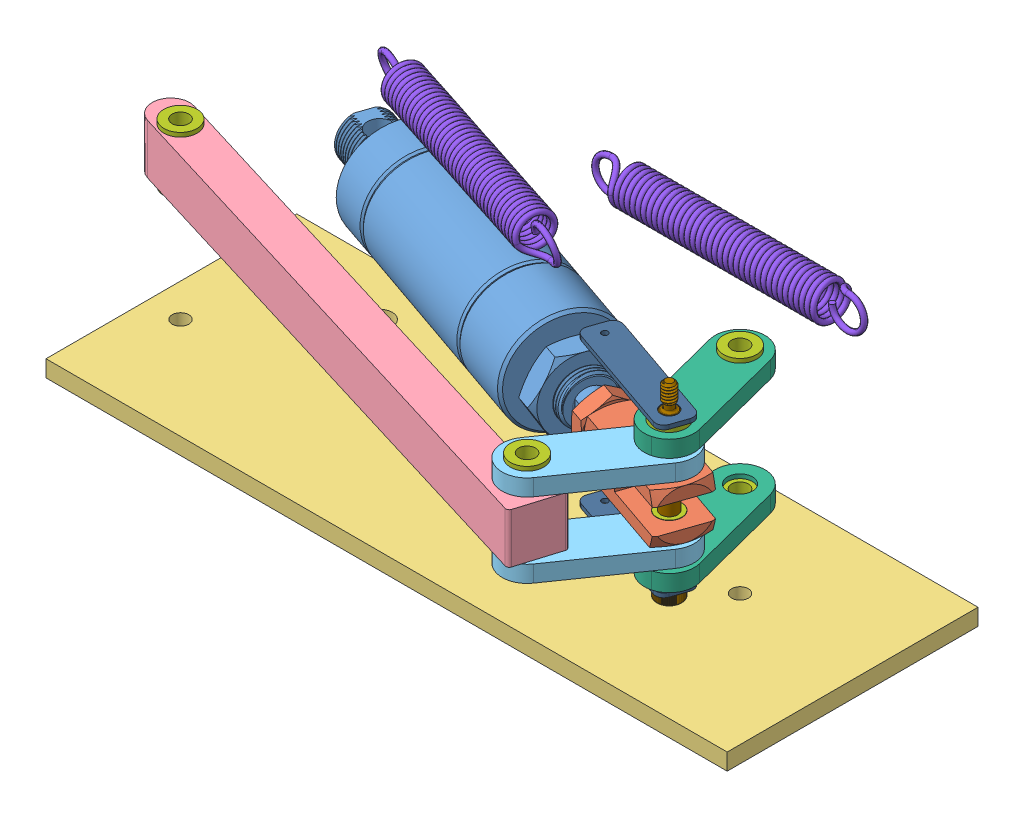
SolidWorks assembly Brake Assembly, configuration Default. Lengths in mm.
Overall size (538.69 101.29 156.86).
28 component instances, 10 part files, 54 mates.
Components (placement in the parent):
- Braking Piston-1: Braking Piston [Default] at (164.5211 173.4692 63.7009) x (-0.945257 0 -0.326326) z (0 -1 0) size (198.34 39.62 39.62) (flexible)
  - Piston for Brakes 6498K983-1: Piston for Brakes 6498K983 [6498K983] at (80.307 95.7083 111.838) size (166.18 39.62 39.62)
  - Brake Piston Rod Clevis 6498K44-1: Brake Piston Rod Clevis 6498K44 [6498K44] at (7.9351 95.7083 111.838) x (0 0 1) z (0 -1 0) size (22 51.06 19.05)
- Brake Mounting Bar-1: Brake Mounting Bar [Default] at (50.8149 0 -76.8043) size (538.69 6.35 114.9)
- Brake Bottom Bar-1: Brake Bottom Bar [Default] at (57.3167 52.1062 -68.9319) x (0.982053 0 0.188604) z (-0.188604 0 0.982053) size (214.1 19.05 36.15)
- Brake Bottom Short Linkage-1: Brake Bottom Short Linkage [Default] at (78.7603 44.1687 -113.4175) x (0.97252 0 0.23282) z (-0.23282 0 0.97252) size (33.27 6.35 55.41)
- Brake Bottom Short Linkage-2: Brake Bottom Short Linkage [Default] at (78.7603 72.7437 -113.4175) x (0.97252 0 0.23282) z (-0.23282 0 0.97252) size (33.27 6.35 55.41)
- Brake Short Top Short Linkage-1: Brake Short Top Short Linkage [Default] at (50.5741 36.2312 -34.9184) x (0.966151 0 -0.257976) z (0.257976 0 0.966151) size (19.38 6.35 56.68)
- Brake Short Top Short Linkage-2: Brake Short Top Short Linkage [Default] at (50.5741 80.6812 -34.9184) x (0.966151 0 -0.257976) z (0.257976 0 0.966151) size (19.38 6.35 56.68)
- Brakes Bronze Bushing-1: Brakes Bronze Bushing [6338K411] at (219.705 72.7437 -18.4994) x (-0.83291 0 -0.553408) z (-0.553408 0 0.83291) size (12.7 6.35 12.7)
- Brakes Bronze Bushing-2: Brakes Bronze Bushing [6338K411] at (219.705 50.5187 -18.4994) size (12.7 6.35 12.7)
- Brakes Bronze Bushing-3: Brakes Bronze Bushing [6338K411] at (197.4073 72.7437 13.5493) x (0.840037 0 0.542529) z (0.542529 0 -0.840037) size (12.7 6.35 12.7)
- Brakes Bronze Bushing-4: Brakes Bronze Bushing [6338K411] at (197.4073 50.5187 13.5493) x (0.999992 0 -0.00402) z (0.00402 0 0.999992) size (12.7 6.35 12.7)
- Brakes Bronze Bushing-5: Brakes Bronze Bushing [6338K411] at (219.705 80.6812 -18.4994) x (-0.837169 0 -0.546944) z (-0.546944 0 0.837169) size (12.7 6.35 12.7)
- Brakes Bronze Bushing-6: Brakes Bronze Bushing [6338K411] at (219.705 42.5812 -18.4994) size (12.7 6.35 12.7)
- Brakes Bronze Bushing-7: Brakes Bronze Bushing [6338K411] at (210.3103 34.6437 -54.9436) size (12.7 6.35 12.7)
- Brakes Bronze Bushing-8: Brakes Bronze Bushing [6338K411] at (219.705 88.6187 -18.4994) x (-0.891229 0 -0.453553) z (-0.453553 0 0.891229) size (12.7 6.35 12.7)
- Brakes Bronze Bushing-9: Brakes Bronze Bushing [6338K411] at (210.3103 88.6187 -54.9436) x (-0.837169 0 -0.546944) z (-0.546944 0 0.837169) size (12.7 6.35 12.7)
- Brakes Bronze Bushing-10: Brakes Bronze Bushing [6338K411] at (219.705 34.6437 -18.4994) x (0.965083 0 -0.261946) z (0.261946 0 0.965083) size (12.7 6.35 12.7)
- Brakes Bronze Bushing-12: Brakes Bronze Bushing [6338K411] at (12.7 50.5187 -38.7043) x (0.988051 0 -0.154127) z (0.154127 0 0.988051) size (12.7 6.35 12.7)
- Brakes Bronze Bushing-13: Brakes Bronze Bushing [6338K411] at (12.7 72.7437 -38.7043) x (-0.837169 0 -0.546944) z (-0.546944 0 0.837169) size (12.7 6.35 12.7)
- Brakes Bronze Bushing-14: Brakes Bronze Bushing [6338K411] at (197.4073 80.6812 13.5493) x (-0.983904 0 -0.178699) z (-0.178699 0 0.983904) size (12.7 6.35 12.7)
- Brakes Bronze Bushing-15: Brakes Bronze Bushing [6338K411] at (197.4073 42.5812 13.5493) size (12.7 6.35 12.7)
- Brakes Return Spring-1: Brakes Return Spring [9654K324] at (100.1802 92.2599 -61.7232) x (0.952226 -0.005044 0.305352) z (0.296812 0.250647 -0.921455) size (104.77 14.45 14.71)
- Brakes Return Spring-2: Brakes Return Spring [9654K324] at (140.1667 54.0208 -121.1624) size (104.77 14.45 14.71)
- Brakes Piston Head Pivot Bolt-1: Brakes Piston Head Pivot Bolt [91259A104] at (219.705 33.0562 -18.4994) x (-0.730056 0 -0.683388) z (-0.683388 0 0.730056) size (9.53 71.79 9.53)
- Brakes Brake Extensions-1: Brakes Brake Extensions [Default] at (179.7604 90.2062 -39.007) x (0.945257 0 0.326326) z (0.326326 0 -0.945257) size (50.8 1.59 12.7)
- Brakes Brake Extensions-2: Brakes Brake Extensions [Default] at (175.6161 33.0562 -27.0022) x (0.945257 0 0.326326) z (-0.326326 0 0.945257) size (50.8 1.59 12.7)
Mates (geometry in assembly coordinates):
- Coincident5: coincident aligned: plane of Brake Mounting Bar-1 through (0 6.35 0) normal (0 0 1); plane of assembly through (0 0 0) normal (0 0 1)
- Coincident6: coincident anti-aligned: plane of Brake Mounting Bar-1 through (50.8149 0 -76.8043) normal (0 -1 0); plane of assembly through (0 0 0) normal (0 1 0)
- Coincident7: coincident anti-aligned: plane of Brake Mounting Bar-1 through (0 6.35 -95.8543) normal (-1 0 0); plane of assembly through (0 0 0) normal (1 0 0)
- Concentric3: concentric anti-aligned: cylinder of Braking Piston-1/Piston for Brakes 6498K983-1 through (50.8149 71.1562 -76.8043) axis (0 -1 0) radius 4.7625; cylinder of Brake Mounting Bar-1 through (50.8149 0 -76.8043) axis (0 1 0) radius 4.7625
- Concentric4: concentric aligned: cylinder of Brake Mounting Bar-1 through (12.7 0 -38.7043) axis (0 1 0) radius 3.175; cylinder of Brake Bottom Bar-1 through (12.7 52.1062 -38.7043) axis (0 1 0) radius 4.7625
- Concentric5: concentric aligned: cylinder of Brake Bottom Short Linkage-2 through (219.705 79.0937 -18.4994) axis (0 -1 0) radius 4.7625; cylinder of Braking Piston-1/Brake Piston Rod Clevis 6498K44-1 through (219.705 71.1562 -18.4994) axis (0 -1 0) radius 4.826
- Concentric6: concentric aligned: cylinder of Braking Piston-1/Brake Piston Rod Clevis 6498K44-1 through (219.705 71.1562 -18.4994) axis (0 -1 0) radius 4.826; cylinder of Brake Bottom Short Linkage-1 through (219.705 50.5187 -18.4994) axis (0 -1 0) radius 4.7625
- Concentric7: concentric anti-aligned: cylinder of Brake Bottom Bar-1 through (197.4073 52.1062 13.5493) axis (0 1 0) radius 4.7625; cylinder of Brake Bottom Short Linkage-1 through (197.4073 50.5187 13.5493) axis (0 -1 0) radius 4.7625
- Concentric8: concentric anti-aligned: cylinder of Brake Bottom Bar-1 through (197.4073 52.1062 13.5493) axis (0 1 0) radius 4.7625; cylinder of Brake Bottom Short Linkage-2 through (197.4073 79.0937 13.5493) axis (0 -1 0) radius 4.7625
- Concentric9: concentric aligned: cylinder of Braking Piston-1/Brake Piston Rod Clevis 6498K44-1 through (219.705 71.1562 -18.4994) axis (0 -1 0) radius 4.826; cylinder of Brake Short Top Short Linkage-2 through (219.705 87.0312 -18.4994) axis (0 -1 0) radius 4.7625
- Concentric10: concentric aligned: cylinder of Braking Piston-1/Brake Piston Rod Clevis 6498K44-1 through (219.705 71.1562 -18.4994) axis (0 -1 0) radius 4.826; cylinder of Brake Short Top Short Linkage-1 through (219.705 42.5812 -18.4994) axis (0 -1 0) radius 4.7625
- Concentric11: concentric anti-aligned: cylinder of Brake Mounting Bar-1 through (210.3103 0 -54.9436) axis (0 1 0) radius 3.175; cylinder of Brake Short Top Short Linkage-1 through (210.3103 42.5812 -54.9436) axis (0 -1 0) radius 4.7625
- Concentric12: concentric anti-aligned: cylinder of Brake Mounting Bar-1 through (210.3103 0 -54.9436) axis (0 1 0) radius 3.175; cylinder of Brake Short Top Short Linkage-2 through (210.3103 87.0312 -54.9436) axis (0 -1 0) radius 4.7625
- Concentric13: concentric anti-aligned: cylinder of Braking Piston-1/Brake Piston Rod Clevis 6498K44-1 through (219.705 71.1562 -18.4994) axis (0 -1 0) radius 4.826; cylinder of Brakes Bronze Bushing-1 through (219.705 66.3937 -18.4994) axis (0 1 0) radius 4.7625
- Coincident15: coincident anti-aligned: plane of Braking Piston-1/Brake Piston Rod Clevis 6498K44-1 through (185.1442 71.1562 -20.354) normal (0 1 0); plane of Brakes Bronze Bushing-1 through (219.705 71.1562 -18.4994) normal (0 -1 0)
- Coincident16: coincident anti-aligned: plane of Braking Piston-1/Brake Piston Rod Clevis 6498K44-1 through (185.1442 52.1062 -20.354) normal (0 -1 0); plane of Brakes Bronze Bushing-2 through (219.705 52.1062 -18.4994) normal (0 1 0)
- Concentric14: concentric aligned: cylinder of Braking Piston-1/Brake Piston Rod Clevis 6498K44-1 through (219.705 71.1562 -18.4994) axis (0 -1 0) radius 4.826; cylinder of Brakes Bronze Bushing-2 through (219.705 56.8687 -18.4994) axis (0 -1 0) radius 3.2004
- Concentric15: concentric aligned: cylinder of Brake Bottom Short Linkage-1 through (219.705 50.5187 -18.4994) axis (0 -1 0) radius 4.7625; cylinder of Brakes Bronze Bushing-6 through (219.705 48.9312 -18.4994) axis (0 -1 0) radius 4.7625
- Coincident17: coincident anti-aligned: plane of Brake Bottom Short Linkage-1 through (78.7603 44.1687 -113.4175) normal (0 -1 0); plane of Brakes Bronze Bushing-6 through (219.705 44.1687 -18.4994) normal (0 1 0)
- Concentric16: concentric aligned: cylinder of Brake Short Top Short Linkage-1 through (219.705 42.5812 -18.4994) axis (0 -1 0) radius 4.7625; cylinder of Brakes Bronze Bushing-10 through (219.705 40.9937 -18.4994) axis (0 -1 0) radius 4.7625
- Coincident19: coincident anti-aligned: plane of Brakes Bronze Bushing-10 through (219.705 36.2312 -18.4994) normal (0 1 0); plane of Brake Short Top Short Linkage-1 through (50.5741 36.2312 -34.9184) normal (0 -1 0)
- Coincident20: coincident anti-aligned: plane of Brake Bottom Short Linkage-2 through (78.7603 79.0937 -113.4175) normal (0 1 0); plane of Brakes Bronze Bushing-5 through (219.705 79.0937 -18.4994) normal (0 -1 0)
- Concentric17: concentric anti-aligned: cylinder of Brake Bottom Short Linkage-2 through (219.705 79.0937 -18.4994) axis (0 -1 0) radius 4.7625; cylinder of Brakes Bronze Bushing-5 through (219.705 74.3312 -18.4994) axis (0 1 0) radius 3.2004
- Concentric18: concentric anti-aligned: cylinder of Brake Short Top Short Linkage-2 through (219.705 87.0312 -18.4994) axis (0 -1 0) radius 4.7625; cylinder of Brakes Bronze Bushing-8 through (219.705 82.2687 -18.4994) axis (0 1 0) radius 4.7625
- Coincident21: coincident anti-aligned: plane of Brake Short Top Short Linkage-2 through (50.5741 87.0312 -34.9184) normal (0 1 0); plane of Brakes Bronze Bushing-8 through (219.705 87.0312 -18.4994) normal (0 -1 0)
- Concentric19: concentric anti-aligned: cylinder of Brake Short Top Short Linkage-2 through (210.3103 87.0312 -54.9436) axis (0 -1 0) radius 4.7625; cylinder of Brakes Bronze Bushing-9 through (210.3103 82.2687 -54.9436) axis (0 1 0) radius 4.7625
- Coincident22: coincident anti-aligned: plane of Brake Short Top Short Linkage-2 through (50.5741 87.0312 -34.9184) normal (0 1 0); plane of Brakes Bronze Bushing-9 through (210.3103 87.0312 -54.9436) normal (0 -1 0)
- Concentric20: concentric aligned: cylinder of Brake Short Top Short Linkage-1 through (210.3103 42.5812 -54.9436) axis (0 -1 0) radius 4.7625; cylinder of Brakes Bronze Bushing-7 through (210.3103 40.9937 -54.9436) axis (0 -1 0) radius 4.7625
- Coincident23: coincident anti-aligned: plane of Brake Short Top Short Linkage-1 through (50.5741 36.2312 -34.9184) normal (0 -1 0); plane of Brakes Bronze Bushing-7 through (210.3103 36.2312 -54.9436) normal (0 1 0)
- Concentric25: concentric anti-aligned: cylinder of Brake Bottom Bar-1 through (12.7 52.1062 -38.7043) axis (0 1 0) radius 4.7625; cylinder of Brakes Bronze Bushing-12 through (12.7 56.8687 -38.7043) axis (0 -1 0) radius 4.7625
- Coincident27: coincident anti-aligned: plane of Brake Bottom Bar-1 through (57.3167 52.1062 -68.9319) normal (0 -1 0); plane of Brakes Bronze Bushing-12 through (12.7 52.1062 -38.7043) normal (0 1 0)
- Concentric26: concentric aligned: cylinder of Brake Bottom Bar-1 through (12.7 52.1062 -38.7043) axis (0 1 0) radius 4.7625; cylinder of Brakes Bronze Bushing-13 through (12.7 66.3937 -38.7043) axis (0 1 0) radius 4.7625
- Coincident28: coincident anti-aligned: plane of Brake Bottom Bar-1 through (57.3167 71.1562 -68.9319) normal (0 1 0); plane of Brakes Bronze Bushing-13 through (12.7 71.1562 -38.7043) normal (0 -1 0)
- Coincident29: coincident anti-aligned: plane of Brake Bottom Short Linkage-1 through (78.7603 50.5187 -113.4175) normal (0 1 0); plane of Brakes Bronze Bushing-2 through (219.705 50.5187 -18.4994) normal (0 -1 0)
- Coincident30: coincident anti-aligned: plane of Brake Short Top Short Linkage-1 through (50.5741 42.5812 -34.9184) normal (0 1 0); plane of Brakes Bronze Bushing-6 through (219.705 42.5812 -18.4994) normal (0 -1 0)
- Coincident31: coincident anti-aligned: plane of Brake Bottom Short Linkage-2 through (78.7603 72.7437 -113.4175) normal (0 -1 0); plane of Brakes Bronze Bushing-1 through (219.705 72.7437 -18.4994) normal (0 1 0)
- Coincident32: coincident anti-aligned: plane of Brake Short Top Short Linkage-2 through (50.5741 80.6812 -34.9184) normal (0 -1 0); plane of Brakes Bronze Bushing-5 through (219.705 80.6812 -18.4994) normal (0 1 0)
- Coincident38: coincident anti-aligned: plane of Brake Bottom Bar-1 through (57.3167 71.1562 -68.9319) normal (0 1 0); plane of Brakes Bronze Bushing-3 through (197.4073 71.1562 13.5493) normal (0 -1 0)
- Concentric27: concentric aligned: cylinder of Brake Bottom Bar-1 through (197.4073 52.1062 13.5493) axis (0 1 0) radius 4.7625; cylinder of Brakes Bronze Bushing-3 through (197.4073 66.3937 13.5493) axis (0 1 0) radius 4.7625
- Concentric28: concentric anti-aligned: cylinder of Brake Bottom Bar-1 through (197.4073 52.1062 13.5493) axis (0 1 0) radius 4.7625; cylinder of Brakes Bronze Bushing-4 through (197.4073 56.8687 13.5493) axis (0 -1 0) radius 3.2004
- Coincident39: coincident anti-aligned: plane of Brake Bottom Bar-1 through (57.3167 52.1062 -68.9319) normal (0 -1 0); plane of Brakes Bronze Bushing-4 through (197.4073 52.1062 13.5493) normal (0 1 0)
- Coincident40: coincident anti-aligned: plane of Brake Bottom Short Linkage-2 through (78.7603 72.7437 -113.4175) normal (0 -1 0); plane of Brakes Bronze Bushing-3 through (197.4073 72.7437 13.5493) normal (0 1 0)
- Concentric29: concentric anti-aligned: cylinder of Brake Bottom Short Linkage-2 through (197.4073 79.0937 13.5493) axis (0 -1 0) radius 4.7625; cylinder of Brakes Bronze Bushing-14 through (197.4073 74.3312 13.5493) axis (0 1 0) radius 4.7625
- Coincident41: coincident anti-aligned: plane of Brake Bottom Short Linkage-2 through (78.7603 79.0937 -113.4175) normal (0 1 0); plane of Brakes Bronze Bushing-14 through (197.4073 79.0937 13.5493) normal (0 -1 0)
- Concentric30: concentric aligned: cylinder of Brake Bottom Short Linkage-1 through (197.4073 50.5187 13.5493) axis (0 -1 0) radius 4.7625; cylinder of Brakes Bronze Bushing-15 through (197.4073 48.9312 13.5493) axis (0 -1 0) radius 4.7625
- Coincident42: coincident anti-aligned: plane of Brake Bottom Short Linkage-1 through (78.7603 44.1687 -113.4175) normal (0 -1 0); plane of Brakes Bronze Bushing-15 through (197.4073 44.1687 13.5493) normal (0 1 0)
- Concentric31: concentric aligned: cylinder of Brakes Bronze Bushing-8 through (219.705 82.2687 -18.4994) axis (0 1 0) radius 3.2004; cylinder of Brakes Piston Head Pivot Bolt-1 through (219.705 33.0562 -18.4994) axis (0 1 0) radius 3.175
- Coincident45: coincident anti-aligned: plane of Brakes Bronze Bushing-8 through (219.705 88.6187 -18.4994) normal (0 1 0); plane of Brakes Brake Extensions-1 through (179.7604 88.6187 -39.007) normal (0 -1 0)
- Concentric33: concentric anti-aligned: cylinder of Brakes Bronze Bushing-8 through (219.705 82.2687 -18.4994) axis (0 1 0) radius 3.2004; cylinder of Brakes Brake Extensions-1 through (219.705 90.2062 -18.4994) axis (0 -1 0) radius 3.175
- Parallel3: parallel aligned: plane of Braking Piston-1/Brake Piston Rod Clevis 6498K44-1 through (231.9368 71.1562 -24.3533) normal (0.326326 0 -0.945257); plane of Brakes Brake Extensions-1 through (179.7604 88.6187 -39.007) normal (0.326326 0 -0.945257)
- Coincident47: coincident anti-aligned: plane of Brakes Bronze Bushing-10 through (219.705 34.6437 -18.4994) normal (0 -1 0); plane of Brakes Brake Extensions-2 through (175.6161 34.6437 -27.0022) normal (0 1 0)
- Concentric34: concentric anti-aligned: cylinder of Brakes Bronze Bushing-10 through (219.705 36.2312 -18.4994) axis (0 -1 0) radius 6.35; cylinder of Brakes Brake Extensions-2 through (219.705 33.0562 -18.4994) axis (0 1 0) radius 3.175
- Coincident48: coincident aligned: plane of Brakes Brake Extensions-1 through (179.7604 88.6187 -39.007) normal (0.326326 0 -0.945257); plane of Brakes Brake Extensions-2 through (179.7604 34.6437 -39.007) normal (0.326326 0 -0.945257)
- Coincident49: coincident anti-aligned: plane of Brakes Piston Head Pivot Bolt-1 through (219.705 33.0562 -18.4994) normal (0 1 0); plane of Brakes Brake Extensions-2 through (175.6161 33.0562 -27.0022) normal (0 -1 0)
